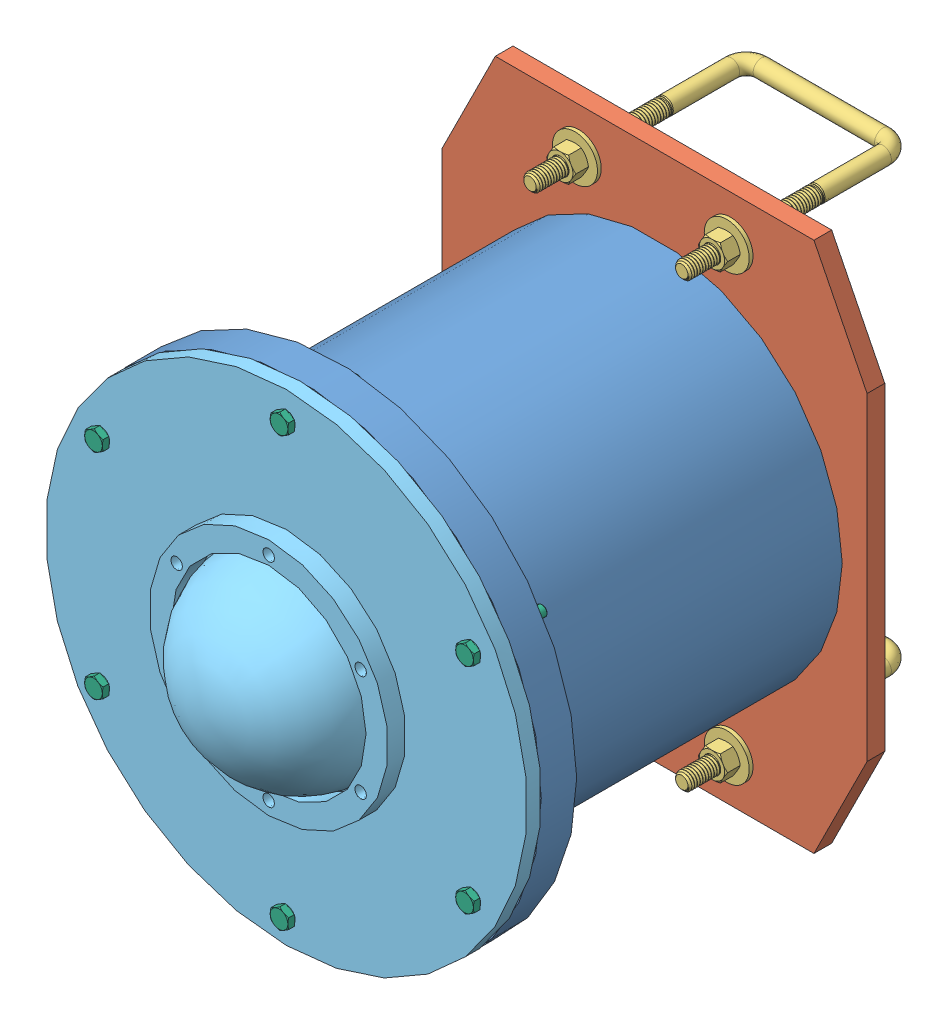
SolidWorks assembly Photogrametry_V2, configuration Default. Lengths in mm.
Overall size (272 300 465).
28 component instances, 10 part files, 36 mates.
Components (placement in the parent):
- Custom_Cylinder_v2-1: Custom_Cylinder_v2 [Default] at (0 0 10) size (272 272 200)
- Back Plate_V2-1: Back Plate_V2 [Default] at origin size (240 300 210)
- 3060T850_SQUARE U-BOLT-1: 3060T850_SQUARE U-BOLT [3060T85] at (0 -125 37.5336) x (-1 0 0) z (0 1 0) size (111.12 127.82 25.4)
- 3060T850_SQUARE U-BOLT-2: 3060T850_SQUARE U-BOLT [3060T85] at (0 125 37.5336) x (-1 0 0) z (0 1 0) size (111.12 127.82 25.4)
- O-ring 210mm-1: O-ring 210mm [1302N432] at (-1.179 1.8509 206.8689) size (222 222 6)
- Custom Dome_v2.1-2: Custom Dome_v2.1 [Default] at (0 0 210) x (1 0 0) z (0 -1 0) size (272 55 272)
- hex cap screw_am-2: hex cap screw_am [B18.2.3.1M - Hex cap screw, M6 x 1.0 x 40 --18N] at (-104.7891 60.5 222.15) x (0 0 -1) z (1 0 0) size (44.15 11.55 10)
- hex cap screw_am-3: hex cap screw_am [B18.2.3.1M - Hex cap screw, M6 x 1.0 x 40 --18N] at (0 121 222.15) x (0 0 -1) z (1 0 0) size (44.15 11.55 10)
- hex cap screw_am-4: hex cap screw_am [B18.2.3.1M - Hex cap screw, M6 x 1.0 x 40 --18N] at (104.7891 60.5 222.15) x (0 0 -1) z (1 0 0) size (44.15 11.55 10)
- hex cap screw_am-5: hex cap screw_am [B18.2.3.1M - Hex cap screw, M6 x 1.0 x 40 --18N] at (104.7891 -60.5 222.15) x (0 0 -1) z (1 0 0) size (44.15 11.55 10)
- hex cap screw_am-6: hex cap screw_am [B18.2.3.1M - Hex cap screw, M6 x 1.0 x 40 --18N] at (0 -121 222.15) x (0 0 -1) z (1 0 0) size (44.15 11.55 10)
- hex cap screw_am-7: hex cap screw_am [B18.2.3.1M - Hex cap screw, M6 x 1.0 x 40 --18N] at (-104.7891 -60.5 222.15) x (0 0 -1) z (1 0 0) size (44.15 11.55 10)
- hex nut jam_am-2: hex nut jam_am [B18.2.4.5M - Hex jam nut,  M6 x 1 --D-N] at (104.7891 60.5 190.4658) size (10 11.55 3.2)
- hex nut jam_am-3: hex nut jam_am [B18.2.4.5M - Hex jam nut,  M6 x 1 --D-N] at (0 121 190.6396) size (10 11.55 3.2)
- hex nut jam_am-4: hex nut jam_am [B18.2.4.5M - Hex jam nut,  M6 x 1 --D-N] at (104.7891 -60.5 190.2875) size (10 11.55 3.2)
- hex nut jam_am-5: hex nut jam_am [B18.2.4.5M - Hex jam nut,  M6 x 1 --D-N] at (0 -121 189.1944) size (10 11.55 3.2)
- hex nut jam_am-6: hex nut jam_am [B18.2.4.5M - Hex jam nut,  M6 x 1 --D-N] at (-104.7891 -60.5 187.2147) size (10 11.55 3.2)
- hex nut jam_am-7: hex nut jam_am [B18.2.4.5M - Hex jam nut,  M6 x 1 --D-N] at (-104.7891 60.5 186.2072) size (10 11.55 3.2)
- camera case V3-1: camera case V3 [Default] at (0 0 108.5989) x (0.999771 -0.021416 0) z (0 0 1) size (200 200 92)
- BOLT M8x100mm-1: BOLT M8x100mm [91180A559] at (48.9445 -49.8096 69.791) x (0 0 -1) z (0.999965 -0.008363 0) size (105.71 15.01 13)
- BOLT M8x100mm-2: BOLT M8x100mm [91180A559] at (-51.0326 -47.668 70.5108) x (0 0 -1) z (0.957019 -0.290025 0) size (105.71 15.01 13)
- BOLT M8x100mm-3: BOLT M8x100mm [91180A559] at (1.4991 69.9839 69.9968) x (0 0 -1) z (0.966642 0.256132 0) size (105.71 15.01 13)
- ROD M8 150mm-1: ROD M8 150mm [98861A593] at (18.1028 -49.7493 120.0995) x (-0.017452 0 -0.999848) z (0.999848 0 -0.017452) size (76.44 8.14 9.24)
- ROD M8 150mm-2: ROD M8 150mm [98861A593] at (16.794 -49.7493 45.1199) x (-0.017452 0 -0.999848) z (0.999848 0 -0.017452) size (76.44 8.14 9.24)
- ROD M8 150mm-5: ROD M8 150mm [98861A593] at (-21.5492 -47.6194 49.405) x (0 0 -1) z (1 0 0) size (76.44 8.14 9.24)
- ROD M8 150mm-6: ROD M8 150mm [98861A593] at (-21.5492 -47.6194 124.396) x (0 0 -1) z (1 0 0) size (76.44 8.14 9.24)
- hex nut jam_am-9: hex nut jam_am [B18.2.4.5M - Hex jam nut,  M8 x 1.25 --D-N] at (23.4706 71.9484 22.7121) size (13 15.01 4)
- hex nut jam_am-10: hex nut jam_am [B18.2.4.5M - Hex jam nut,  M8 x 1.25 --D-N] at (60.5193 -46.2227 22.6039) size (13 15.01 4)
Mates (geometry in assembly coordinates):
- Concentric1: concentric: cylinder of Back Plate_V2-1 through (0 0 0) axis (0 0 -1); cylinder of Custom_Cylinder_v2-1 through (0 0 210) axis (0 0 -1) radius 101
- Coincident2: coincident: plane of Back Plate_V2-1 through (0 0 10) normal (0 0 1); plane of Custom_Cylinder_v2-1 through (0 0 10) normal (0 0 -1)
- Concentric6: concentric aligned: cylinder of Custom_Cylinder_v2-1 through (0 0 210) axis (0 0 -1) radius 106; line of Back Plate_V2-1 through (0 0 0) axis (0 0 -1)
- Coincident7: coincident anti-aligned: plane of Custom_Cylinder_v2-1 through (0 0 10) normal (0 0 -1); plane of Back Plate_V2-1 through (0 0 10) normal (0 0 1)
- Concentric7: concentric anti-aligned: cylinder of Back Plate_V2-1 through (42.8625 -125 10) axis (0 0 -1) radius 7.5; cylinder of 3060T850_SQUARE U-BOLT-1 through (42.8625 -125 -76.1314) axis (0 0 1) radius 4.7625
- Concentric8: concentric anti-aligned: cylinder of Back Plate_V2-1 through (42.8625 125 10) axis (0 0 -1) radius 7.5; cylinder of 3060T850_SQUARE U-BOLT-2 through (42.8625 125 -76.1314) axis (0 0 1) radius 4.7625
- Coincident8: coincident anti-aligned: plane of Back Plate_V2-1 through (0 0 10) normal (0 0 1); plane of 3060T850_SQUARE U-BOLT-2 through (-42.8625 125 10) normal (0 0 -1)
- Coincident9: coincident anti-aligned: plane of Back Plate_V2-1 through (0 0 10) normal (0 0 1); plane of 3060T850_SQUARE U-BOLT-1 through (-42.8625 -125 10) normal (0 0 -1)
- Coincident13: coincident anti-aligned: circle of Custom_Cylinder_v2-1; circle of Custom Dome_v2.1-2
- Coincident14: coincident anti-aligned: circle of Custom_Cylinder_v2-1; circle of Custom Dome_v2.1-2
- Concentric11: concentric anti-aligned: cylinder of Custom Dome_v2.1-2 through (-104.7891 60.5 232) axis (0 0 -1) radius 3.3; cylinder of hex cap screw_am-2 through (-104.7891 60.5 222.15) axis (0 0 1) radius 3
- Coincident17: coincident anti-aligned: plane of Custom Dome_v2.1-2 through (0 0 218) normal (0 0 1); plane of hex cap screw_am-2 through (-104.7891 66.2735 218) normal (0 0 -1)
- Concentric12: concentric anti-aligned: cylinder of Custom Dome_v2.1-2 through (0 121 232) axis (0 0 -1) radius 3.3; cylinder of hex cap screw_am-3 through (0 121 222.15) axis (0 0 1) radius 3
- Coincident18: coincident anti-aligned: plane of Custom Dome_v2.1-2 through (0 0 218) normal (0 0 1); plane of hex cap screw_am-3 through (0 126.7735 218) normal (0 0 -1)
- Concentric13: concentric anti-aligned: cylinder of Custom Dome_v2.1-2 through (104.7891 60.5 232) axis (0 0 -1) radius 3.3; cylinder of hex cap screw_am-4 through (104.7891 60.5 222.15) axis (0 0 1) radius 3
- Coincident19: coincident anti-aligned: plane of Custom Dome_v2.1-2 through (0 0 218) normal (0 0 1); plane of hex cap screw_am-4 through (104.7891 66.2735 218) normal (0 0 -1)
- Concentric14: concentric anti-aligned: cylinder of Custom Dome_v2.1-2 through (104.7891 -60.5 232) axis (0 0 -1) radius 3.3; cylinder of hex cap screw_am-5 through (104.7891 -60.5 222.15) axis (0 0 1) radius 3
- Coincident20: coincident anti-aligned: plane of Custom Dome_v2.1-2 through (0 0 218) normal (0 0 1); plane of hex cap screw_am-5 through (104.7891 -54.7265 218) normal (0 0 -1)
- Concentric15: concentric anti-aligned: cylinder of Custom Dome_v2.1-2 through (0 -121 232) axis (0 0 -1) radius 3.3; cylinder of hex cap screw_am-6 through (0 -121 222.15) axis (0 0 1) radius 3
- Coincident21: coincident anti-aligned: plane of Custom Dome_v2.1-2 through (0 0 218) normal (0 0 1); plane of hex cap screw_am-6 through (0 -115.2265 218) normal (0 0 -1)
- Concentric16: concentric anti-aligned: cylinder of Custom Dome_v2.1-2 through (-104.7891 -60.5 232) axis (0 0 -1) radius 3.3; cylinder of hex cap screw_am-7 through (-104.7891 -60.5 222.15) axis (0 0 1) radius 3
- Coincident22: coincident anti-aligned: plane of Custom Dome_v2.1-2 through (0 0 218) normal (0 0 1); plane of hex cap screw_am-7 through (-104.7891 -54.7265 218) normal (0 0 -1)
- Concentric17: concentric aligned: cylinder of hex cap screw_am-4 through (104.7891 60.5 222.15) axis (0 0 1) radius 3; cylinder of hex nut jam_am-2 through (104.7891 60.5 165.4283) axis (0 0 1) radius 3
- Concentric18: concentric aligned: cylinder of hex cap screw_am-3 through (0 121 222.15) axis (0 0 1) radius 3; cylinder of hex nut jam_am-3 through (0 121 165.6021) axis (0 0 1) radius 3
- Concentric19: concentric aligned: cylinder of hex cap screw_am-5 through (104.7891 -60.5 222.15) axis (0 0 1) radius 3; cylinder of hex nut jam_am-4 through (104.7891 -60.5 165.25) axis (0 0 1) radius 3
- Concentric20: concentric aligned: cylinder of hex cap screw_am-6 through (0 -121 222.15) axis (0 0 1) radius 3; cylinder of hex nut jam_am-5 through (0 -121 164.1568) axis (0 0 1) radius 3
- Concentric21: concentric aligned: cylinder of hex cap screw_am-7 through (-104.7891 -60.5 222.15) axis (0 0 1) radius 3; cylinder of hex nut jam_am-6 through (-104.7891 -60.5 162.1772) axis (0 0 1) radius 3
- Concentric22: concentric aligned: cylinder of hex cap screw_am-2 through (-104.7891 60.5 222.15) axis (0 0 1) radius 3; cylinder of hex nut jam_am-7 through (-104.7891 60.5 161.1697) axis (0 0 1) radius 3
- Concentric23: concentric anti-aligned: cylinder of Custom_Cylinder_v2-1 through (0 0 210) axis (0 0 -1) radius 106; cylinder of camera case V3-1 through (0 0 73.5989) axis (0 0 1) radius 33.75
- Concentric27: concentric anti-aligned: circle of camera case V3-1; cylinder of BOLT M8x100mm-1 through (48.9445 -49.8096 117.141) axis (0 0 -1) radius 4
- Concentric28: concentric anti-aligned: circle of camera case V3-1; cylinder of BOLT M8x100mm-2 through (-51.0326 -47.668 117.8608) axis (0 0 -1) radius 4
- Concentric30: concentric aligned: circle of camera case V3-1; cylinder of BOLT M8x100mm-3 through (1.4991 69.9839 117.3468) axis (0 0 -1) radius 4
- Concentric34: concentric anti-aligned: circle of ROD M8 150mm-1; circle of ROD M8 150mm-2
- Lock1: lock: unknown of ROD M8 150mm-1; unknown of ROD M8 150mm-2
- Concentric37: concentric anti-aligned: circle of ROD M8 150mm-5; circle of ROD M8 150mm-6
- Lock2: lock: unknown of ROD M8 150mm-5; unknown of ROD M8 150mm-6
